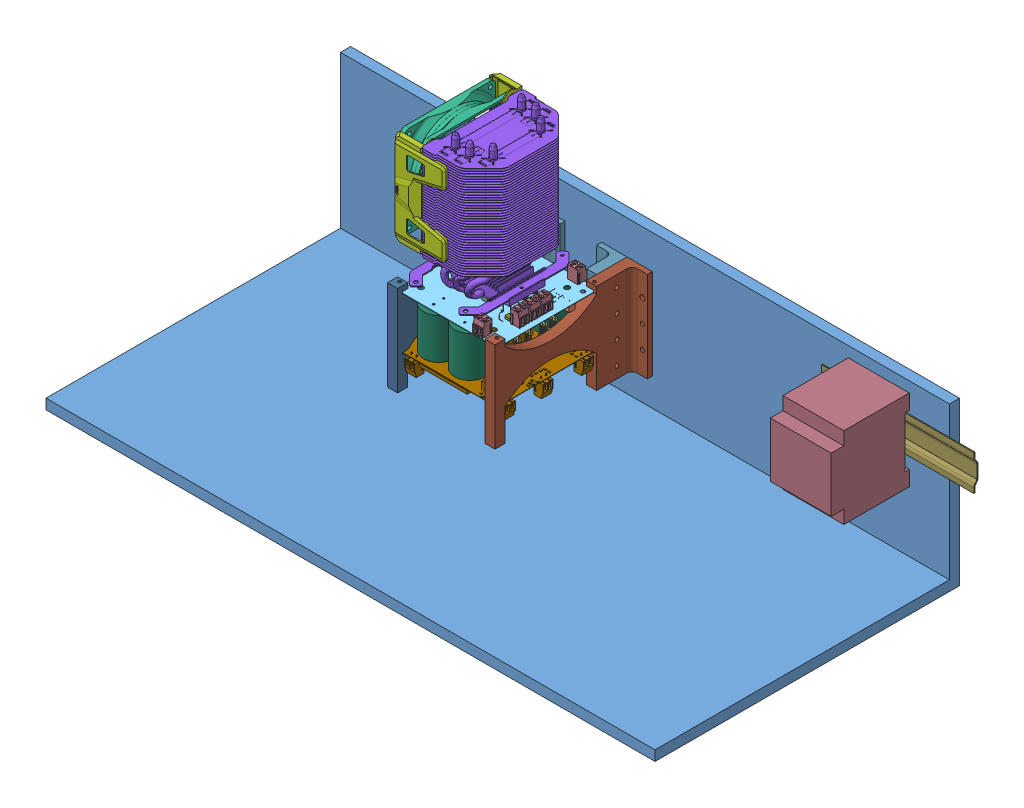
SolidWorks assembly Assem227, configuration Default. Lengths in mm.
Overall size (628.12 265.72 300).
337 component instances, 34 part files, 13 mates.
Components (placement in the parent):
- estrutura_madeira-1: estrutura_madeira [Default] at (156.2068 160.4481 379.7942) size (600 160 300)
- conversor-1: conversor [Default] at (101.5779 266.6814 325.8895) x (-1 0 0) z (0 1 0) size (196.64 140 240.72)
  - inversor_rev2-1: inversor_rev2 [Default] at (-42.011 -49.0953 13.8297) size (100.07 109.25 61.05)
    - inversor_rev2.step-1: inversor_rev2.step [Default] at origin size (100.07 109.25 61.05)
      - R11.step-1: R11.step [Default] at origin size (1.4 2.15 0.65)
        - 1052595968.step-1: 1052595968.step [Default] at (72.136 29.972 0) size (1.4 2.15 0.65)
          - Extruded.step-1: Extruded.step [Default] at origin size (1.4 2.15 0.65)
      - R10.step-1: R10.step [Default] at origin size (1.4 2.15 0.65)
        - 1052595968.step-1: 1052595968.step [Default] at (74.93 29.972 0) size (1.4 2.15 0.65)
          - Extruded.step-1: Extruded.step [Default] at origin size (1.4 2.15 0.65)
      - P8.step-1: P8.step [Default] at origin size (7.72 2.67 47.1)
        - zl201-3_p2-54_l7-62_w2-54_h8-89.step-1: zl201-3_p2-54_l7-62_w2-54_h8-89.step [Default] at (83.5661 26.6699 -43.4013) x (1 0 0) z (0 -1 0) size (7.62 11.94 2.54)
        - zl201-3_p2-54_l7-62_w2-54_h8-89.step-2: zl201-3_p2-54_l7-62_w2-54_h8-89.step [Default] at (83.6675 26.7717 -20) x (1 0 0) z (0 -1 0) size (7.62 11.94 2.54)
        - zl201-3_p2-54_l7-62_w2-54_h8-89.step-3: zl201-3_p2-54_l7-62_w2-54_h8-89.step [Default] at (83.6675 26.7717 -2.4013) x (1 0 0) z (0 1 0) size (7.62 11.94 2.54)
        - zl201-3_p2-54_l7-62_w2-54_h8-89.step-4: zl201-3_p2-54_l7-62_w2-54_h8-89.step [Default] at (83.6675 26.7971 -31.9013) x (1 0 0) z (0 -1 0) size (7.62 11.94 2.54)
      - C19.step-1: C19.step [Default] at origin size (1.45 2.2 1.1)
        - 1052595832.step-1: 1052595832.step [Default] at (83.566 21.59 0) size (1.45 2.2 1.1)
          - Extruded-4.step-1: Extruded-4.step [Default] at origin size (1.45 2.2 1.1)
      - C18.step-1: C18.step [Default] at origin size (1.45 2.2 1.1)
        - 1052595832.step-1: 1052595832.step [Default] at (69.342 30.353 0) size (1.45 2.2 1.1)
          - Extruded-4.step-1: Extruded-4.step [Default] at origin size (1.45 2.2 1.1)
      - C11.step-1: C11.step [Default] at origin size (3.4 1.8 1.35)
        - 1052596240.step-1: 1052596240.step [Default] at (79.502 24.892 -1.7513) size (3.4 1.8 1.35)
          - Extruded-1.step-1: Extruded-1.step [Default] at origin size (3.4 1.8 1.35)
      - C10.step-1: C10.step [Default] at origin size (4.3 7.5 4)
        - 1052596648.step-1: 1052596648.step [Default] at (79.502 22.352 0) size (4.3 4.9 4)
          - Extruded-2.step-1: Extruded-2.step [Default] at origin size (4.3 4.9 4)
        - 1052596784.step-1: 1052596784.step [Default] at (79.502 19.252 0) size (4.3 1.3 4)
          - Extruded-3.step-1: Extruded-3.step [Default] at origin size (4.3 1.3 4)
        - 1052596784.step-2: 1052596784.step [Default] at (79.502 25.452 0) size (4.3 1.3 4)
          - Extruded-3.step-1: Extruded-3.step [Default] at origin size (4.3 1.3 4)
      - C22.step-1: C22.step [Default] at origin size (1.45 2.2 1.1)
        - 1052597056.step-1: 1052597056.step [Default] at (74.93 32.512 -1.7513) size (1.45 2.2 1.1)
          - Extruded-4.step-1: Extruded-4.step [Default] at origin size (1.45 2.2 1.1)
      - C21.step-1: C21.step [Default] at origin size (4.3 7.5 4)
        - 1052596648.step-1: 1052596648.step [Default] at (79.502 31.242 0) size (4.3 4.9 4)
          - Extruded-2.step-1: Extruded-2.step [Default] at origin size (4.3 4.9 4)
        - 1052596784.step-1: 1052596784.step [Default] at (79.502 28.142 0) size (4.3 1.3 4)
          - Extruded-3.step-1: Extruded-3.step [Default] at origin size (4.3 1.3 4)
        - 1052596784.step-2: 1052596784.step [Default] at (79.502 34.342 0) size (4.3 1.3 4)
          - Extruded-3.step-1: Extruded-3.step [Default] at origin size (4.3 1.3 4)
      - C20.step-1: C20.step [Default] at origin size (4.3 7.5 4)
        - 1052596648.step-1: 1052596648.step [Default] at (79.248 31.242 -4.4013) size (4.3 4.9 4)
          - Extruded-2.step-1: Extruded-2.step [Default] at origin size (4.3 4.9 4)
        - 1052596784.step-1: 1052596784.step [Default] at (79.248 28.142 -4.4013) size (4.3 1.3 4)
          - Extruded-3.step-1: Extruded-3.step [Default] at origin size (4.3 1.3 4)
        - 1052596784.step-2: 1052596784.step [Default] at (79.248 34.342 -4.4013) size (4.3 1.3 4)
          - Extruded-3.step-1: Extruded-3.step [Default] at origin size (4.3 1.3 4)
      - D3.step-1: D3.step [Default] at origin size (20 1.52 1.52)
        - do35_d1-5_l3.step-1: do35_d1-5_l3.step [Default] at (49.9079 33.2429 -1.4013) x (1 0 0) z (0 0 -1) size (20 1.52 1.52)
          - Open CASCADE STEP translator 6.8 1.12.1.1.step-1: Open CASCADE STEP translator 6.8 1.12.1.1.step [Default] at origin size (20 1.52 1.52)
          - Open CASCADE STEP translator 6.8 1.12.1.2.step-1: Open CASCADE STEP translator 6.8 1.12.1.2.step [Default] at origin
      - D2.step-1: D2.step [Default] at origin size (20 1.52 1.52)
        - do35_d1-5_l3.step-1: do35_d1-5_l3.step [Default] at (49.9619 38.0745 -1.4013) x (1 0 0) z (0 0 -1) size (20 1.52 1.52)
          - Open CASCADE STEP translator 6.8 1.12.1.1.step-1: Open CASCADE STEP translator 6.8 1.12.1.1.step [Default] at origin size (20 1.52 1.52)
          - Open CASCADE STEP translator 6.8 1.12.1.2.step-1: Open CASCADE STEP translator 6.8 1.12.1.2.step [Default] at origin
      - D1.step-1: D1.step [Default] at origin size (20 1.52 1.52)
        - do35_d1-5_l3.step-1: do35_d1-5_l3.step [Default] at (49.9959 42.6465 -1.4013) x (1 0 0) z (0 0 -1) size (20 1.52 1.52)
          - Open CASCADE STEP translator 6.8 1.12.1.1.step-1: Open CASCADE STEP translator 6.8 1.12.1.1.step [Default] at origin size (20 1.52 1.52)
          - Open CASCADE STEP translator 6.8 1.12.1.2.step-1: Open CASCADE STEP translator 6.8 1.12.1.2.step [Default] at origin
      - R13.step-1: R13.step [Default] at origin size (2.15 1.4 0.65)
        - 1052596104.step-1: 1052596104.step [Default] at (58.928 35.56 -1.0513) size (2.15 1.4 0.65)
          - Extruded-5.step-1: Extruded-5.step [Default] at origin size (2.15 1.4 0.65)
      - R15.step-1: R15.step [Default] at origin size (2.15 1.4 0.65)
        - 1052596104.step-1: 1052596104.step [Default] at (40.132 33.782 -1.0513) size (2.15 1.4 0.65)
          - Extruded-5.step-1: Extruded-5.step [Default] at origin size (2.15 1.4 0.65)
      - R14.step-1: R14.step [Default] at origin size (2.15 1.4 0.65)
        - 1052596104.step-1: 1052596104.step [Default] at (40.386 38.608 -1.0513) size (2.15 1.4 0.65)
          - Extruded-5.step-1: Extruded-5.step [Default] at origin size (2.15 1.4 0.65)
      - R12.step-1: R12.step [Default] at origin size (2.15 1.4 0.65)
        - 1052596104.step-1: 1052596104.step [Default] at (40.386 43.434 -1.0513) size (2.15 1.4 0.65)
          - Extruded-5.step-1: Extruded-5.step [Default] at origin size (2.15 1.4 0.65)
      - C26.step-1: C26.step [Default] at origin size (2.2 1.45 1.1)
        - 1052596920.step-1: 1052596920.step [Default] at (41.402 40.64 -1.5013) size (2.2 1.45 1.1)
          - Extruded-6.step-1: Extruded-6.step [Default] at origin size (2.2 1.45 1.1)
      - C25.step-1: C25.step [Default] at origin size (2.2 1.45 1.1)
        - 1052596920.step-1: 1052596920.step [Default] at (41.402 35.814 -1.5013) size (2.2 1.45 1.1)
          - Extruded-6.step-1: Extruded-6.step [Default] at origin size (2.2 1.45 1.1)
      - C24.step-1: C24.step [Default] at origin size (2.2 1.45 1.1)
        - 1052596920.step-1: 1052596920.step [Default] at (41.402 30.988 -1.5013) size (2.2 1.45 1.1)
          - Extruded-6.step-1: Extruded-6.step [Default] at origin size (2.2 1.45 1.1)
      - R17.step-1: R17.step [Default] at origin size (1.4 2.15 0.65)
        - 1052595968.step-1: 1052595968.step [Default] at (78.994 14.478 0) size (1.4 2.15 0.65)
          - Extruded.step-1: Extruded.step [Default] at origin size (1.4 2.15 0.65)
      - P1.step-1: P1.step [Default] at origin size (7.72 2.67 47.1)
        - zl201-3_p2-54_l7-62_w2-54_h8-89.step-1: zl201-3_p2-54_l7-62_w2-54_h8-89.step [Default] at (83.5661 34.2899 -43.4013) x (1 0 0) z (0 -1 0) size (7.62 11.94 2.54)
        - zl201-3_p2-54_l7-62_w2-54_h8-89.step-2: zl201-3_p2-54_l7-62_w2-54_h8-89.step [Default] at (83.6675 34.3917 -20) x (1 0 0) z (0 -1 0) size (7.62 11.94 2.54)
        - zl201-3_p2-54_l7-62_w2-54_h8-89.step-3: zl201-3_p2-54_l7-62_w2-54_h8-89.step [Default] at (83.6675 34.3917 -2.4013) x (1 0 0) z (0 1 0) size (7.62 11.94 2.54)
        - zl201-3_p2-54_l7-62_w2-54_h8-89.step-4: zl201-3_p2-54_l7-62_w2-54_h8-89.step [Default] at (83.6675 34.4171 -31.9013) x (1 0 0) z (0 -1 0) size (7.62 11.94 2.54)
      - C17.step-1: C17.step [Default] at origin size (2.2 1.45 1.1)
        - 1052596920.step-1: 1052596920.step [Default] at (75.946 47.498 -1.5013) size (2.2 1.45 1.1)
          - Extruded-6.step-1: Extruded-6.step [Default] at origin size (2.2 1.45 1.1)
      - C16.step-1: C16.step [Default] at origin size (2.2 1.45 1.1)
        - 1052596920.step-1: 1052596920.step [Default] at (75.946 41.402 -1.5013) size (2.2 1.45 1.1)
          - Extruded-6.step-1: Extruded-6.step [Default] at origin size (2.2 1.45 1.1)
      - C15.step-1: C15.step [Default] at origin size (2.2 1.45 1.1)
        - 1052596920.step-1: 1052596920.step [Default] at (75.946 45.466 -1.5013) size (2.2 1.45 1.1)
          - Extruded-6.step-1: Extruded-6.step [Default] at origin size (2.2 1.45 1.1)
      - C14.step-1: C14.step [Default] at origin size (2.2 1.45 1.1)
        - 1052596920.step-1: 1052596920.step [Default] at (75.946 39.37 -1.5013) size (2.2 1.45 1.1)
          - Extruded-6.step-1: Extruded-6.step [Default] at origin size (2.2 1.45 1.1)
      - C13.step-1: C13.step [Default] at origin size (2.2 1.45 1.1)
        - 1052596920.step-1: 1052596920.step [Default] at (75.946 43.434 -1.5013) size (2.2 1.45 1.1)
          - Extruded-6.step-1: Extruded-6.step [Default] at origin size (2.2 1.45 1.1)
      - C12.step-1: C12.step [Default] at origin size (2.2 1.45 1.1)
        - 1052596920.step-1: 1052596920.step [Default] at (75.946 37.338 -1.5013) size (2.2 1.45 1.1)
          - Extruded-6.step-1: Extruded-6.step [Default] at origin size (2.2 1.45 1.1)
      - P2.step-1: P2.step [Default] at origin size (7.72 2.67 47.1)
        - zl201-3_p2-54_l7-62_w2-54_h8-89.step-1: zl201-3_p2-54_l7-62_w2-54_h8-89.step [Default] at (83.5661 47.4979 -43.4013) x (1 0 0) z (0 -1 0) size (7.62 11.94 2.54)
        - zl201-3_p2-54_l7-62_w2-54_h8-89.step-2: zl201-3_p2-54_l7-62_w2-54_h8-89.step [Default] at (83.6675 47.5997 -20) x (1 0 0) z (0 -1 0) size (7.62 11.94 2.54)
        - zl201-3_p2-54_l7-62_w2-54_h8-89.step-3: zl201-3_p2-54_l7-62_w2-54_h8-89.step [Default] at (83.6675 47.5997 -2.4013) x (1 0 0) z (0 1 0) size (7.62 11.94 2.54)
        - zl201-3_p2-54_l7-62_w2-54_h8-89.step-4: zl201-3_p2-54_l7-62_w2-54_h8-89.step [Default] at (83.6675 47.6251 -31.9013) x (1 0 0) z (0 -1 0) size (7.62 11.94 2.54)
      - P3.step-1: P3.step [Default] at origin size (7.72 2.67 47.1)
        - zl201-3_p2-54_l7-62_w2-54_h8-89.step-1: zl201-3_p2-54_l7-62_w2-54_h8-89.step [Default] at (83.5661 41.5289 -43.4013) x (1 0 0) z (0 -1 0) size (7.62 11.94 2.54)
        - zl201-3_p2-54_l7-62_w2-54_h8-89.step-2: zl201-3_p2-54_l7-62_w2-54_h8-89.step [Default] at (83.6675 41.6307 -20) x (1 0 0) z (0 -1 0) size (7.62 11.94 2.54)
        - zl201-3_p2-54_l7-62_w2-54_h8-89.step-3: zl201-3_p2-54_l7-62_w2-54_h8-89.step [Default] at (83.6675 41.6307 -2.4013) x (1 0 0) z (0 1 0) size (7.62 11.94 2.54)
        - zl201-3_p2-54_l7-62_w2-54_h8-89.step-4: zl201-3_p2-54_l7-62_w2-54_h8-89.step [Default] at (83.6675 41.6561 -31.9013) x (1 0 0) z (0 -1 0) size (7.62 11.94 2.54)
      - R6.step-1: R6.step [Default] at origin size (2.15 1.4 0.65)
        - 1052596104.step-1: 1052596104.step [Default] at (75.946 37.338 0) size (2.15 1.4 0.65)
          - Extruded-5.step-1: Extruded-5.step [Default] at origin size (2.15 1.4 0.65)
      - R5.step-1: R5.step [Default] at origin size (2.15 1.4 0.65)
        - 1052596104.step-1: 1052596104.step [Default] at (75.946 39.37 0) size (2.15 1.4 0.65)
          - Extruded-5.step-1: Extruded-5.step [Default] at origin size (2.15 1.4 0.65)
      - R4.step-1: R4.step [Default] at origin size (2.15 1.4 0.65)
        - 1052596104.step-1: 1052596104.step [Default] at (75.946 41.402 0) size (2.15 1.4 0.65)
          - Extruded-5.step-1: Extruded-5.step [Default] at origin size (2.15 1.4 0.65)
      - R3.step-1: R3.step [Default] at origin size (2.15 1.4 0.65)
        - 1052596104.step-1: 1052596104.step [Default] at (75.946 43.434 0) size (2.15 1.4 0.65)
          - Extruded-5.step-1: Extruded-5.step [Default] at origin size (2.15 1.4 0.65)
      - R2.step-1: R2.step [Default] at origin size (2.15 1.4 0.65)
        - 1052596104.step-1: 1052596104.step [Default] at (75.946 45.466 0) size (2.15 1.4 0.65)
          - Extruded-5.step-1: Extruded-5.step [Default] at origin size (2.15 1.4 0.65)
      - R1.step-1: R1.step [Default] at origin size (2.15 1.4 0.65)
        - 1052596104.step-1: 1052596104.step [Default] at (75.946 47.498 0) size (2.15 1.4 0.65)
          - Extruded-5.step-1: Extruded-5.step [Default] at origin size (2.15 1.4 0.65)
      - C8.step-1: C8.step [Default] at origin size (7.5 4.3 4)
        - 1052596376.step-1: 1052596376.step [Default] at (75.211 51.816 0) size (4.9 4.3 4)
          - Extruded-7.step-1: Extruded-7.step [Default] at origin size (4.9 4.3 4)
        - 1052596512.step-1: 1052596512.step [Default] at (72.111 51.816 0) size (1.3 4.3 4)
          - Extruded-8.step-1: Extruded-8.step [Default] at origin size (1.3 4.3 4)
        - 1052596512.step-2: 1052596512.step [Default] at (78.311 51.816 0) size (1.3 4.3 4)
          - Extruded-8.step-1: Extruded-8.step [Default] at origin size (1.3 4.3 4)
      - C6.step-1: C6.step [Default] at origin size (7.5 4.3 4)
        - 1052596376.step-1: 1052596376.step [Default] at (71.855 58.928 0) size (4.9 4.3 4)
          - Extruded-7.step-1: Extruded-7.step [Default] at origin size (4.9 4.3 4)
        - 1052596512.step-1: 1052596512.step [Default] at (74.955 58.928 0) size (1.3 4.3 4)
          - Extruded-8.step-1: Extruded-8.step [Default] at origin size (1.3 4.3 4)
        - 1052596512.step-2: 1052596512.step [Default] at (68.755 58.928 0) size (1.3 4.3 4)
          - Extruded-8.step-1: Extruded-8.step [Default] at origin size (1.3 4.3 4)
      - C4.step-1: C4.step [Default] at origin size (7.5 4.3 4)
        - 1052596376.step-1: 1052596376.step [Default] at (72.136 65.786 0) size (4.9 4.3 4)
          - Extruded-7.step-1: Extruded-7.step [Default] at origin size (4.9 4.3 4)
        - 1052596512.step-1: 1052596512.step [Default] at (75.236 65.786 0) size (1.3 4.3 4)
          - Extruded-8.step-1: Extruded-8.step [Default] at origin size (1.3 4.3 4)
        - 1052596512.step-2: 1052596512.step [Default] at (69.036 65.786 0) size (1.3 4.3 4)
          - Extruded-8.step-1: Extruded-8.step [Default] at origin size (1.3 4.3 4)
      - -VDC1.step-1: -VDC1.step [Default] at origin size (10.6 9 17)
        - SCREW_TERMINAL_BLOCK_5MM.step-1: SCREW_TERMINAL_BLOCK_5MM.step [Default] at (20.1591 6.4347 2) x (-1 0 0) z (0 1 0) size (10.6 17 9)
      - +VDC1.step-1: +VDC1.step [Default] at origin size (10.6 9 17)
        - SCREW_TERMINAL_BLOCK_5MM.step-1: SCREW_TERMINAL_BLOCK_5MM.step [Default] at (10.9959 90.0853 2) x (1 0 0) z (0 -1 0) size (10.6 17 9)
      - P7.step-1: P7.step [Default] at origin size (7.72 2.67 47.1)
        - zl201-3_p2-54_l7-62_w2-54_h8-89.step-1: zl201-3_p2-54_l7-62_w2-54_h8-89.step [Default] at (18.0339 26.1621 -43.4013) x (-1 0 0) z (0 1 0) size (7.62 11.94 2.54)
        - zl201-3_p2-54_l7-62_w2-54_h8-89.step-2: zl201-3_p2-54_l7-62_w2-54_h8-89.step [Default] at (17.9325 26.0603 -20) x (-1 0 0) z (0 1 0) size (7.62 11.94 2.54)
        - zl201-3_p2-54_l7-62_w2-54_h8-89.step-3: zl201-3_p2-54_l7-62_w2-54_h8-89.step [Default] at (17.9325 26.0603 -2.4013) x (-1 0 0) z (0 -1 0) size (7.62 11.94 2.54)
        - zl201-3_p2-54_l7-62_w2-54_h8-89.step-4: zl201-3_p2-54_l7-62_w2-54_h8-89.step [Default] at (17.9325 26.0349 -31.9013) x (-1 0 0) z (0 1 0) size (7.62 11.94 2.54)
      - P6.step-1: P6.step [Default] at origin size (7.72 2.67 47.1)
        - zl201-3_p2-54_l7-62_w2-54_h8-89.step-1: zl201-3_p2-54_l7-62_w2-54_h8-89.step [Default] at (18.0339 35.8141 -43.4013) x (-1 0 0) z (0 1 0) size (7.62 11.94 2.54)
        - zl201-3_p2-54_l7-62_w2-54_h8-89.step-2: zl201-3_p2-54_l7-62_w2-54_h8-89.step [Default] at (17.9325 35.7123 -20) x (-1 0 0) z (0 1 0) size (7.62 11.94 2.54)
        - zl201-3_p2-54_l7-62_w2-54_h8-89.step-3: zl201-3_p2-54_l7-62_w2-54_h8-89.step [Default] at (17.9325 35.7123 -2.4013) x (-1 0 0) z (0 -1 0) size (7.62 11.94 2.54)
        - zl201-3_p2-54_l7-62_w2-54_h8-89.step-4: zl201-3_p2-54_l7-62_w2-54_h8-89.step [Default] at (17.9325 35.6869 -31.9013) x (-1 0 0) z (0 1 0) size (7.62 11.94 2.54)
      - P5.step-1: P5.step [Default] at origin size (7.72 2.67 47.1)
        - zl201-3_p2-54_l7-62_w2-54_h8-89.step-1: zl201-3_p2-54_l7-62_w2-54_h8-89.step [Default] at (18.0339 50.0381 -43.4013) x (-1 0 0) z (0 1 0) size (7.62 11.94 2.54)
        - zl201-3_p2-54_l7-62_w2-54_h8-89.step-2: zl201-3_p2-54_l7-62_w2-54_h8-89.step [Default] at (17.9325 49.9363 -20) x (-1 0 0) z (0 1 0) size (7.62 11.94 2.54)
        - zl201-3_p2-54_l7-62_w2-54_h8-89.step-3: zl201-3_p2-54_l7-62_w2-54_h8-89.step [Default] at (17.9325 49.9363 -2.4013) x (-1 0 0) z (0 -1 0) size (7.62 11.94 2.54)
        - zl201-3_p2-54_l7-62_w2-54_h8-89.step-4: zl201-3_p2-54_l7-62_w2-54_h8-89.step [Default] at (17.9325 49.9109 -31.9013) x (-1 0 0) z (0 1 0) size (7.62 11.94 2.54)
      - P4.step-1: P4.step [Default] at origin size (7.72 2.67 47.1)
        - zl201-3_p2-54_l7-62_w2-54_h8-89.step-1: zl201-3_p2-54_l7-62_w2-54_h8-89.step [Default] at (18.0339 61.9761 -43.4013) x (-1 0 0) z (0 1 0) size (7.62 11.94 2.54)
        - zl201-3_p2-54_l7-62_w2-54_h8-89.step-2: zl201-3_p2-54_l7-62_w2-54_h8-89.step [Default] at (17.9325 61.8743 -20) x (-1 0 0) z (0 1 0) size (7.62 11.94 2.54)
        - zl201-3_p2-54_l7-62_w2-54_h8-89.step-3: zl201-3_p2-54_l7-62_w2-54_h8-89.step [Default] at (17.9325 61.8743 -2.4013) x (-1 0 0) z (0 -1 0) size (7.62 11.94 2.54)
        - zl201-3_p2-54_l7-62_w2-54_h8-89.step-4: zl201-3_p2-54_l7-62_w2-54_h8-89.step [Default] at (17.9325 61.8489 -31.9013) x (-1 0 0) z (0 1 0) size (7.62 11.94 2.54)
      - W1.step-1: W1.step [Default] at origin size (9 10.6 17)
        - SCREW_TERMINAL_BLOCK_5MM.step-1: SCREW_TERMINAL_BLOCK_5MM.step [Default] at (10.4987 39.4909 2) x (0 1 0) z (1 0 0) size (10.6 17 9)
      - V1.step-1: V1.step [Default] at origin size (9 10.6 17)
        - SCREW_TERMINAL_BLOCK_5MM.step-1: SCREW_TERMINAL_BLOCK_5MM.step [Default] at (10.4987 50.9209 2) x (0 1 0) z (1 0 0) size (10.6 17 9)
      - U1.step-1: U1.step [Default] at origin size (9 10.6 17)
        - SCREW_TERMINAL_BLOCK_5MM.step-1: SCREW_TERMINAL_BLOCK_5MM.step [Default] at (10.4987 62.3509 2) x (0 1 0) z (1 0 0) size (10.6 17 9)
      - C3.step-1: C3.step [Default] at origin size (3.4 1.8 1.35)
        - 1052596240.step-1: 1052596240.step [Default] at (16.51 52.578 -1.7513) size (3.4 1.8 1.35)
          - Extruded-1.step-1: Extruded-1.step [Default] at origin size (3.4 1.8 1.35)
      - C2.step-1: C2.step [Default] at origin size (3.4 1.8 1.35)
        - 1052596240.step-1: 1052596240.step [Default] at (16.637 64.516 -1.7513) size (3.4 1.8 1.35)
          - Extruded-1.step-1: Extruded-1.step [Default] at origin size (3.4 1.8 1.35)
      - C1.step-1: C1.step [Default] at origin size (3.4 1.8 1.35)
        - 1052596240.step-1: 1052596240.step [Default] at (16.51 38.354 -1.7513) size (3.4 1.8 1.35)
          - Extruded-1.step-1: Extruded-1.step [Default] at origin size (3.4 1.8 1.35)
      - U2.step-1: U2.step [Default] at origin size (29.83 36.3 7.7)
        - User_Library-Cipos-mini-PCB.step-1: User_Library-Cipos-mini-PCB.step [Default] at (38.058 67.0707 2.5987) x (0 1 0) z (1 0 0) size (36.3 7.7 29.83)
      - C7.step-1: C7.step [Default] at origin size (7.5 4.3 4)
        - 1052596376.step-1: 1052596376.step [Default] at (72.136 58.928 -4.4013) size (4.9 4.3 4)
          - Extruded-7.step-1: Extruded-7.step [Default] at origin size (4.9 4.3 4)
        - 1052596512.step-1: 1052596512.step [Default] at (75.236 58.928 -4.4013) size (1.3 4.3 4)
          - Extruded-8.step-1: Extruded-8.step [Default] at origin size (1.3 4.3 4)
        - 1052596512.step-2: 1052596512.step [Default] at (69.036 58.928 -4.4013) size (1.3 4.3 4)
          - Extruded-8.step-1: Extruded-8.step [Default] at origin size (1.3 4.3 4)
      - C5.step-1: C5.step [Default] at origin size (7.5 4.3 4)
        - 1052596376.step-1: 1052596376.step [Default] at (71.882 65.786 -4.4013) size (4.9 4.3 4)
          - Extruded-7.step-1: Extruded-7.step [Default] at origin size (4.9 4.3 4)
        - 1052596512.step-1: 1052596512.step [Default] at (74.982 65.786 -4.4013) size (1.3 4.3 4)
          - Extruded-8.step-1: Extruded-8.step [Default] at origin size (1.3 4.3 4)
        - 1052596512.step-2: 1052596512.step [Default] at (68.782 65.786 -4.4013) size (1.3 4.3 4)
          - Extruded-8.step-1: Extruded-8.step [Default] at origin size (1.3 4.3 4)
      - C9.step-1: C9.step [Default] at origin size (7.5 4.3 4)
        - 1052596376.step-1: 1052596376.step [Default] at (75.184 51.562 -4.4013) size (4.9 4.3 4)
          - Extruded-7.step-1: Extruded-7.step [Default] at origin size (4.9 4.3 4)
        - 1052596512.step-1: 1052596512.step [Default] at (72.084 51.562 -4.4013) size (1.3 4.3 4)
          - Extruded-8.step-1: Extruded-8.step [Default] at origin size (1.3 4.3 4)
        - 1052596512.step-2: 1052596512.step [Default] at (78.284 51.562 -4.4013) size (1.3 4.3 4)
          - Extruded-8.step-1: Extruded-8.step [Default] at origin size (1.3 4.3 4)
      - C_bus2.step-1: C_bus2.step [Default] at origin size (30 30 40)
        - 1152675632.step-1: 1152675632.step [Default] at (66.2941 87.0713 -1.4013) x (0 1 0) z (0 0 -1) size (30 30 40)
          - Cylinder.step-1: Cylinder.step [Default] at origin size (30 30 40)
      - C_bus1.step-1: C_bus1.step [Default] at origin size (30 30 40)
        - 1152675632.step-1: 1152675632.step [Default] at (35.5601 87.1221 -1.4013) x (0 1 0) z (0 0 -1) size (30 30 40)
          - Cylinder.step-1: Cylinder.step [Default] at origin size (30 30 40)
      - C_bus4.step-1: C_bus4.step [Default] at origin size (30 30 40)
        - 1152675632.step-1: 1152675632.step [Default] at (35.5601 7.8741 -1.4013) x (0 1 0) z (0 0 -1) size (30 30 40)
          - Cylinder.step-1: Cylinder.step [Default] at origin size (30 30 40)
      - C_bus3.step-1: C_bus3.step [Default] at origin size (30 30 40)
        - 1152675632.step-1: 1152675632.step [Default] at (66.2941 7.8741 -1.4013) x (0 1 0) z (0 0 -1) size (30 30 40)
          - Cylinder.step-1: Cylinder.step [Default] at origin size (30 30 40)
      - CC1.step-1: CC1.step [Default] at origin size (5 3.8 2.55)
        - 1052597192.step-1: 1052597192.step [Default] at (16.6678 67.3928 0.1) size (5 3.8 2.55)
          - Extruded-9.step-1: Extruded-9.step [Default] at origin size (5 3.8 2.55)
      - CC2.step-1: CC2.step [Default] at origin size (5 3.8 2.55)
        - 1052597192.step-1: 1052597192.step [Default] at (16.6678 54.9722 0.1) size (5 3.8 2.55)
          - Extruded-9.step-1: Extruded-9.step [Default] at origin size (5 3.8 2.55)
      - CC3.step-1: CC3.step [Default] at origin size (5 3.8 2.55)
        - 1052597192.step-1: 1052597192.step [Default] at (16.9726 40.9768 0.1) size (5 3.8 2.55)
          - Extruded-9.step-1: Extruded-9.step [Default] at origin size (5 3.8 2.55)
      - C27.step-1: C27.step [Default] at origin size (2.2 1.45 1.1)
        - 1052596920.step-1: 1052596920.step [Default] at (4.572 25.4 -1.5013) size (2.2 1.45 1.1)
          - Extruded-6.step-1: Extruded-6.step [Default] at origin size (2.2 1.45 1.1)
      - C28.step-1: C28.step [Default] at origin size (2.2 1.45 1.1)
        - 1052596920.step-1: 1052596920.step [Default] at (4.572 27.432 -1.5013) size (2.2 1.45 1.1)
          - Extruded-6.step-1: Extruded-6.step [Default] at origin size (2.2 1.45 1.1)
      - C29.step-1: C29.step [Default] at origin size (1.45 2.2 1.1)
        - 1052595832.step-1: 1052595832.step [Default] at (1.778 31.369 -1.5013) size (1.45 2.2 1.1)
          - Extruded-4.step-1: Extruded-4.step [Default] at origin size (1.45 2.2 1.1)
      - C30.step-1: C30.step [Default] at origin size (2.2 1.45 1.1)
        - 1052596920.step-1: 1052596920.step [Default] at (13.716 28.448 0) size (2.2 1.45 1.1)
          - Extruded-6.step-1: Extruded-6.step [Default] at origin size (2.2 1.45 1.1)
      - C31.step-1: C31.step [Default] at origin size (1.45 2.2 1.1)
        - 1052595832.step-1: 1052595832.step [Default] at (18.542 30.734 -1.5013) size (1.45 2.2 1.1)
          - Extruded-4.step-1: Extruded-4.step [Default] at origin size (1.45 2.2 1.1)
      - R7.step-1: R7.step [Default] at origin size (6.65 3.45 0.9)
        - 1152666032.step-1: 1152666032.step [Default] at (28.5496 41.529 0) x (-1 0 0) z (0 0 1) size (6.65 3.45 0.9)
          - Terminal.step-1: Terminal.step [Default] at (-3.325 -1.725 0) size (0.6 3.45 0.9)
            - Open_CASCADE_STEP_translator_6.8_1.2.1.step-1: Open_CASCADE_STEP_translator_6.8_1.2.1.step [Default] at origin size (0.6 3.45 0.9)
          - Terminal.step-2: Terminal.step [Default] at (3.325 1.725 0) x (-1 0 0) z (0 0 1) size (0.6 3.45 0.9)
            - Open_CASCADE_STEP_translator_6.8_1.2.1.step-1: Open_CASCADE_STEP_translator_6.8_1.2.1.step [Default] at origin size (0.6 3.45 0.9)
          - Mid_Body.step-1: Mid_Body.step [Default] at (-3.325 -1.725 0) size (6.47 3.45 0.72)
          - Mark.step-1: Mark.step [Default] at (-2.725 -1.725 0.81) size (5.45 3.45 0.09)
      - R8.step-1: R8.step [Default] at origin size (6.65 3.45 0.9)
        - 1152666032.step-1: 1152666032.step [Default] at (28.5496 36.8808 -0.4013) x (-1 0 0) z (0 0 -1) size (6.65 3.45 0.9)
          - Terminal.step-1: Terminal.step [Default] at (-3.325 -1.725 0) size (0.6 3.45 0.9)
            - Open_CASCADE_STEP_translator_6.8_1.2.1.step-1: Open_CASCADE_STEP_translator_6.8_1.2.1.step [Default] at origin size (0.6 3.45 0.9)
          - Terminal.step-2: Terminal.step [Default] at (3.325 1.725 0) x (-1 0 0) z (0 0 1) size (0.6 3.45 0.9)
            - Open_CASCADE_STEP_translator_6.8_1.2.1.step-1: Open_CASCADE_STEP_translator_6.8_1.2.1.step [Default] at origin size (0.6 3.45 0.9)
          - Mid_Body.step-1: Mid_Body.step [Default] at (-3.325 -1.725 0) size (6.47 3.45 0.72)
          - Mark.step-1: Mark.step [Default] at (-2.725 -1.725 0.81) size (5.45 3.45 0.09)
      - R9.step-1: R9.step [Default] at origin size (6.65 3.45 0.9)
        - 1152666032.step-1: 1152666032.step [Default] at (28.5496 32.3342 0) x (-1 0 0) z (0 0 1) size (6.65 3.45 0.9)
          - Terminal.step-1: Terminal.step [Default] at (-3.325 -1.725 0) size (0.6 3.45 0.9)
            - Open_CASCADE_STEP_translator_6.8_1.2.1.step-1: Open_CASCADE_STEP_translator_6.8_1.2.1.step [Default] at origin size (0.6 3.45 0.9)
          - Terminal.step-2: Terminal.step [Default] at (3.325 1.725 0) x (-1 0 0) z (0 0 1) size (0.6 3.45 0.9)
            - Open_CASCADE_STEP_translator_6.8_1.2.1.step-1: Open_CASCADE_STEP_translator_6.8_1.2.1.step [Default] at origin size (0.6 3.45 0.9)
          - Mid_Body.step-1: Mid_Body.step [Default] at (-3.325 -1.725 0) size (6.47 3.45 0.72)
          - Mark.step-1: Mark.step [Default] at (-2.725 -1.725 0.81) size (5.45 3.45 0.09)
      - R22.step-1: R22.step [Default] at origin size (1.4 2.15 0.65)
        - 1052595968.step-1: 1052595968.step [Default] at (12.7 31.48 0) size (1.4 2.15 0.65)
          - Extruded.step-1: Extruded.step [Default] at origin size (1.4 2.15 0.65)
      - R23.step-1: R23.step [Default] at origin size (1.4 2.15 0.65)
        - 1052595968.step-1: 1052595968.step [Default] at (-0.508 31.369 -1.0513) size (1.4 2.15 0.65)
          - Extruded.step-1: Extruded.step [Default] at origin size (1.4 2.15 0.65)
      - R19.step-1: R19.step [Default] at origin size (1.4 2.15 0.65)
        - 1052595968.step-1: 1052595968.step [Default] at (-0.508 77.268 -1.0513) size (1.4 2.15 0.65)
          - Extruded.step-1: Extruded.step [Default] at origin size (1.4 2.15 0.65)
      - R20.step-1: R20.step [Default] at origin size (1.4 2.15 0.65)
        - 1052595968.step-1: 1052595968.step [Default] at (-0.508 72.95 -1.0513) size (1.4 2.15 0.65)
          - Extruded.step-1: Extruded.step [Default] at origin size (1.4 2.15 0.65)
      - R21.step-1: R21.step [Default] at origin size (1.4 2.15 0.65)
        - 1052595968.step-1: 1052595968.step [Default] at (-0.508 68.632 -1.0513) size (1.4 2.15 0.65)
          - Extruded.step-1: Extruded.step [Default] at origin size (1.4 2.15 0.65)
      - R25.step-1: R25.step [Default] at origin size (1.4 2.15 0.65)
        - 1052595968.step-1: 1052595968.step [Default] at (-0.4698 18.2106 -1.0513) size (1.4 2.15 0.65)
          - Extruded.step-1: Extruded.step [Default] at origin size (1.4 2.15 0.65)
      - R26.step-1: R26.step [Default] at origin size (1.4 2.15 0.65)
        - 1052595968.step-1: 1052595968.step [Default] at (-0.4698 22.5286 -1.0513) size (1.4 2.15 0.65)
          - Extruded.step-1: Extruded.step [Default] at origin size (1.4 2.15 0.65)
      - R27.step-1: R27.step [Default] at origin size (1.4 2.15 0.65)
        - 1052595968.step-1: 1052595968.step [Default] at (-0.4698 26.8466 -1.0513) size (1.4 2.15 0.65)
          - Extruded.step-1: Extruded.step [Default] at origin size (1.4 2.15 0.65)
      - U3.step-1: U3.step [Default] at origin size (15.89 5.82 7)
        - 1052597328.step-1: 1052597328.step [Default] at (8.8002 21.2217 -8.4013) size (15.89 5.82 7)
          - Extruded-10.step-1: Extruded-10.step [Default] at origin size (15.89 5.82 7)
      - U4.step-1: U4.step [Default] at origin size (7.52 5.21 2.8)
        - 1052597736.step-1: 1052597736.step [Default] at (9.525 31.3817 -3.4013) size (7.52 5.21 2.8)
          - Extruded-11.step-1: Extruded-11.step [Default] at origin size (7.52 5.21 2.8)
      - C_bus5.step-1: C_bus5.step [Default] at origin size (7.9 24.84 2)
        - 1052597464.step-1: 1052597464.step [Default] at (22.3139 52.7051 -3.4013) size (7.9 24.84 2)
          - Extruded-12.step-1: Extruded-12.step [Default] at origin size (7.9 24.84 2)
      - R16.step-1: R16.step [Default] at origin size (2.15 1.4 0.65)
        - 1052596104.step-1: 1052596104.step [Default] at (59.436 30.226 -1.0513) size (2.15 1.4 0.65)
          - Extruded-5.step-1: Extruded-5.step [Default] at origin size (2.15 1.4 0.65)
      - C23.step-1: C23.step [Default] at origin size (2.2 1.45 1.1)
        - 1052596920.step-1: 1052596920.step [Default] at (66.548 33.782 -1.5013) size (2.2 1.45 1.1)
          - Extruded-6.step-1: Extruded-6.step [Default] at origin size (2.2 1.45 1.1)
      - R18.step-1: R18.step [Default] at origin size (1.4 2.15 0.65)
        - 1052595968.step-1: 1052595968.step [Default] at (-0.508 81.534 -1.0513) size (1.4 2.15 0.65)
          - Extruded.step-1: Extruded.step [Default] at origin size (1.4 2.15 0.65)
      - R24.step-1: R24.step [Default] at origin size (2.15 1.4 0.65)
        - 1052596104.step-1: 1052596104.step [Default] at (0.508 15.113 -1.0513) size (2.15 1.4 0.65)
          - Extruded-5.step-1: Extruded-5.step [Default] at origin size (2.15 1.4 0.65)
      - Board.step-1: Board.step [Default] at origin size (100.07 99.8 0.41)
  - heatsink-1: heatsink [Default] at (-0.3777 43.1754 102.4783) x (0 -1 0) z (0 0 1) size (108.44 180.01 139.76)
    - 7030025_PART_FAN STANDARD 90_MODEL.igs-1: 7030025_PART_FAN STANDARD 90_MODEL.igs [Default] at (0 45 -45) x (1 0 0) z (0 -1 0) size (93.98 180.01 25.07)
    - 7030026_PART_HEATSINK ADAPTOR 90_MODEL.igs-1: 7030026_PART_HEATSINK ADAPTOR 90_MODEL.igs [Default] at (95 58.5 47.4641) x (0 0 -1) z (-1 0 0) size (106.39 52.6 26.58)
    - 7030026_PART_HEATSINK ADAPTOR 90_MODEL.igs-2: 7030026_PART_HEATSINK ADAPTOR 90_MODEL.igs [Default] at (-7 58.5 -46) x (0 0 1) z (1 0 0) size (106.39 52.6 26.58)
    - 7030027_PART_CPU HEATSINK TOWER_MODEL.igs-1: 7030027_PART_CPU HEATSINK TOWER_MODEL.igs [Default] at (94 31.5 -47.65) x (-1 0 0) z (0 0 1) size (108.44 80.01 139.76)
  - controlo_rev2-1: controlo_rev2 [Default] at (-42.011 -49.0953 -36.5818) size (103.49 101.24 40.41)
  - suporte_topo-1: suporte_topo [Default] at (5.989 -1.0953 -41.2332) x (-1 0 0) z (0 -1 0) size (106 40 100) (hidden)
  - suporte_conversor_frente-3: suporte_conversor_frente [Default] at (48.989 -1.0953 -11.5818) x (0 1 0) z (1 0 0) size (140 89 25)
  - suporte_conversor_trás-1: suporte_conversor_trás [Default] at (-37.011 -1.0953 -11.5818) x (0 -1 0) z (-1 0 0) size (140 89 25)
- calha_din-1: calha_din [Default] at (334.3302 277.318 243.921) x (0 0 1) z (0 1 0) size (4.21 150 35)
- contactor-1: contactor [Default] at (416.6131 270.0423 276.6581) x (0 0 1) z (0 -1 0) size (80 60 80)
- suporte_esquadro-1: suporte_esquadro [Default] at (52.5889 230.0995 324.7942) x (0 0 1) z (1 0 0) size (30 89 25)
- suporte_esquadro-2: suporte_esquadro [Default] at (138.5889 255.0995 324.7942) x (0 0 1) z (-1 0 0) size (30 89 25)
Mates (geometry in assembly coordinates):
- Coincident1: coincident: plane of estrutura_madeira-1 through (-243.7932 370.4481 189.7942) normal (0 0 1); plane of ? through (192.2537 255.0995 189.7942) normal (0 0 -1)
- Distance1: distance = 15 mm: plane of conversor-1/suporte_topo-1 through (95.5889 185.4481 324.7942) normal (0 -1 0); plane of estrutura_madeira-1 through (156.2068 170.4481 379.7942) normal (0 1 0)
- Coincident5: coincident: plane of estrutura_madeira-1 through (-143.7932 320.4481 239.7942) normal (0 0 1); plane of calha_din-1 through (484.3302 270.818 239.7942) normal (0 0 -1)
- Coincident6: coincident: line of calha_din-1 through (484.3302 295.1609 243.921) axis (-1 0 0); line of contactor-1 through (416.6131 295.1609 243.921) axis (-1 0 0)
- Coincident7: coincident: plane of estrutura_madeira-1 through (-143.7932 320.4481 239.7942) normal (0 0 1); plane of conversor-1/suporte_conversor_frente-3 through (52.5889 255.0995 239.7942) normal (0 0 -1)
- Coincident8: coincident: plane of calha_din-1 through (484.3302 265.1609 243.921) normal (0 0 1); plane of contactor-1 through (416.6131 295.1609 243.921) normal (0 0 -1)
- Coincident9: coincident: plane of estrutura_madeira-1 through (-143.7932 320.4481 239.7942) normal (0 0 1); plane of suporte_esquadro-1 through (52.5889 230.0995 239.7942) normal (0 0 -1)
- Coincident11: coincident: plane of conversor-1/suporte_conversor_frente-3 through (52.5889 255.0995 324.7942) normal (1 0 0); plane of suporte_esquadro-1 through (52.5889 230.0995 324.7942) normal (-1 0 0)
- Concentric1: concentric: circle of conversor-1/suporte_conversor_frente-3; circle of suporte_esquadro-1
- Concentric4: concentric: cylinder of conversor-1/suporte_conversor_trás-1 through (138.5889 275.9745 259.7942) axis (1 0 0) radius 2; circle of suporte_esquadro-2
- Coincident18: coincident: plane of conversor-1/suporte_conversor_trás-1 through (138.5889 287.0995 324.7942) normal (0 1 0); plane of suporte_esquadro-2 through (138.5889 287.0995 324.7942) normal (0 1 0)
- Coincident19: coincident: plane of conversor-1/suporte_conversor_trás-1 through (138.5889 255.0995 239.7942) normal (0 0 -1); plane of suporte_esquadro-2 through (138.5889 255.0995 239.7942) normal (0 0 -1)
- Coincident20: coincident: plane of conversor-1/suporte_conversor_trás-1 through (138.5889 255.0995 324.7942) normal (-1 0 0); plane of suporte_esquadro-2 through (138.5889 255.0995 324.7942) normal (1 0 0)
